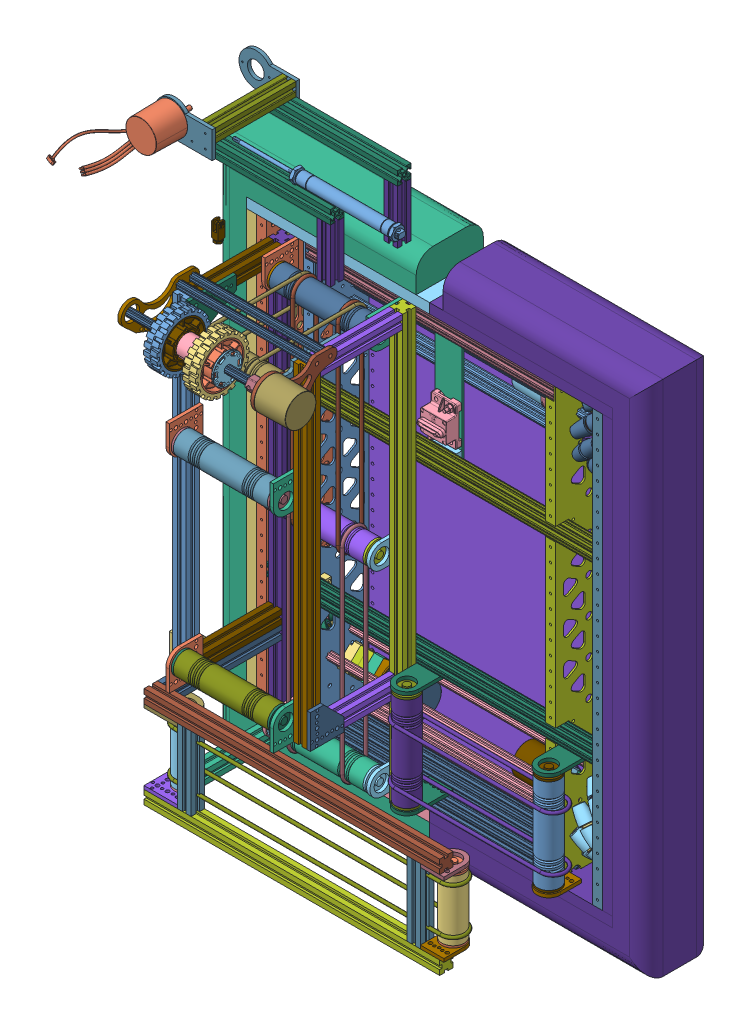
SolidWorks assembly Robot 2020, configuration Default. Lengths in mm. (continued)
Components (placement in the parent): (continued)
- Robot 2020(2)^Robot 2020-1: Robot 2020(2)^Robot 2020 [Default] at origin size (819.15 992.53 549) (virtual) (continued)
  - Fame 2020^Robot 2020(2)_Robot 2020-1: Fame 2020^Robot 2020(2)_Robot 2020 [Default] at origin size (819.15 977.9 171.99) (virtual) (continued)
    - Left Wheel Assembly v4(Mirror)^Fame 2020_Robot 2020(2)_Robot 2020-1: Left Wheel Assembly v4(Mirror)^Fame 2020_Robot 2020(2)_Robot 2020 [Default] at (-500 0 0) x (-1 0 0) z (0 0 -1) size (65.82 166.11 165.01) (virtual) (continued)
      - 6_Mecanum_Wheel_Left_217-2799 v1(Mirror)^Left Wheel Assembly v4(Mirror)_Fame 2020_Robot 2020(2)_Robot 2020-1: 6_Mecanum_Wheel_Left_217-2799 v1(Mirror)^Left Wheel Assembly v4(Mirror)_Fame 2020_Robot 2020(2)_Robot 2020 [Default] x (0 0 -1) z (1 0 0) size (165.01 166.11 65.82) (virtual) (continued)
        - 217-2586-004 Rev1(Mirror)^6_Mecanum_Wheel_Left_217-2799 v1(Mirror)_Left Wheel Assembly v4(Mirror)_Fame 2020_Robot 2020(2)_Robot 2020-6: 217-2586-004 Rev1(Mirror)^6_Mecanum_Wheel_Left_217-2799 v1(Mirror)_Left Wheel Assembly v4(Mirror)_Fame 2020_Robot 2020(2)_Robot 2020 [Default] at (43.5263 -256.0729 -227.2551) x (-0.488796 0.647964 0.584142) z (-0.522795 -0.753596 0.39847) size (25.9 28.58 25.9) (virtual)
        - 217-2586-004 Rev1(Mirror)^6_Mecanum_Wheel_Left_217-2799 v1(Mirror)_Left Wheel Assembly v4(Mirror)_Fame 2020_Robot 2020(2)_Robot 2020-7: 217-2586-004 Rev1(Mirror)^6_Mecanum_Wheel_Left_217-2799 v1(Mirror)_Left Wheel Assembly v4(Mirror)_Fame 2020_Robot 2020(2)_Robot 2020 [Default] at (77.6959 -273.7639 -227.2551) x (-0.01458 0.811521 0.584142) z (-0.865903 -0.302381 0.39847) size (25.9 28.58 25.9) (virtual)
        - 217-2586-004 Rev1(Mirror)^6_Mecanum_Wheel_Left_217-2799 v1(Mirror)_Left Wheel Assembly v4(Mirror)_Fame 2020_Robot 2020(2)_Robot 2020-8: 217-2586-004 Rev1(Mirror)^6_Mecanum_Wheel_Left_217-2799 v1(Mirror)_Left Wheel Assembly v4(Mirror)_Fame 2020_Robot 2020(2)_Robot 2020 [Default] at (94.9412 -308.1606 -227.2551) x (0.465204 0.665104 0.584142) z (-0.878265 0.264334 0.39847) size (25.9 28.58 25.9) (virtual)
        - 217-2586-004 Rev1(Mirror)^6_Mecanum_Wheel_Left_217-2799 v1(Mirror)_Left Wheel Assembly v4(Mirror)_Fame 2020_Robot 2020(2)_Robot 2020-9: 217-2586-004 Rev1(Mirror)^6_Mecanum_Wheel_Left_217-2799 v1(Mirror)_Left Wheel Assembly v4(Mirror)_Fame 2020_Robot 2020(2)_Robot 2020 [Default] at (88.675 -346.1246 -227.2551) x (0.767297 0.26464 0.584142) z (-0.55516 0.730082 0.39847) size (25.9 28.58 25.9) (virtual)
        - 217-2586-004 Rev1(Mirror)^6_Mecanum_Wheel_Left_217-2799 v1(Mirror)_Left Wheel Assembly v4(Mirror)_Fame 2020_Robot 2020(2)_Robot 2020-10: 217-2586-004 Rev1(Mirror)^6_Mecanum_Wheel_Left_217-2799 v1(Mirror)_Left Wheel Assembly v4(Mirror)_Fame 2020_Robot 2020(2)_Robot 2020 [Default] at (61.291 -373.155 -227.2551) x (0.776308 -0.236907 0.584142) z (-0.020002 0.916963 0.39847) size (25.9 28.58 25.9) (virtual)
        - 217-2586-004 Rev1(Mirror)^6_Mecanum_Wheel_Left_217-2799 v1(Mirror)_Left Wheel Assembly v4(Mirror)_Fame 2020_Robot 2020(2)_Robot 2020-11: 217-2586-004 Rev1(Mirror)^6_Mecanum_Wheel_Left_217-2799 v1(Mirror)_Left Wheel Assembly v4(Mirror)_Fame 2020_Robot 2020(2)_Robot 2020 [Default] at (23.2487 -378.9271 -227.2551) x (0.488796 -0.647964 0.584142) z (0.522795 0.753596 0.39847) size (25.9 28.58 25.9) (virtual)
        - 217-2586-004 Rev1(Mirror)^6_Mecanum_Wheel_Left_217-2799 v1(Mirror)_Left Wheel Assembly v4(Mirror)_Fame 2020_Robot 2020(2)_Robot 2020-12: 217-2586-004 Rev1(Mirror)^6_Mecanum_Wheel_Left_217-2799 v1(Mirror)_Left Wheel Assembly v4(Mirror)_Fame 2020_Robot 2020(2)_Robot 2020 [Default] at (-28.0394 -327.6397 -228.0654) x (-0.983582 -0.179 0.02293) z (-0.142587 0.692961 -0.706735) size (25.9 28.58 25.9) (virtual)
        - 217-2586-004 Rev1(Mirror)^6_Mecanum_Wheel_Left_217-2799 v1(Mirror)_Left Wheel Assembly v4(Mirror)_Fame 2020_Robot 2020(2)_Robot 2020-13: 217-2586-004 Rev1(Mirror)^6_Mecanum_Wheel_Left_217-2799 v1(Mirror)_Left Wheel Assembly v4(Mirror)_Fame 2020_Robot 2020(2)_Robot 2020 [Default] at (-22.2679 -289.5974 -228.0654) x (-0.900948 0.433321 0.02293) z (0.291957 0.644427 -0.706735) size (25.9 28.58 25.9) (virtual)
        - 217-2586-004 Rev1(Mirror)^6_Mecanum_Wheel_Left_217-2799 v1(Mirror)_Left Wheel Assembly v4(Mirror)_Fame 2020_Robot 2020(2)_Robot 2020-14: 217-2586-004 Rev1(Mirror)^6_Mecanum_Wheel_Left_217-2799 v1(Mirror)_Left Wheel Assembly v4(Mirror)_Fame 2020_Robot 2020(2)_Robot 2020 [Default] at (4.7621 -262.2129 -228.0654) x (-0.474183 0.880128 0.02293) z (0.614983 0.349745 -0.706735) size (25.9 28.58 25.9) (virtual)
        - 217-2586-004 Rev1(Mirror)^6_Mecanum_Wheel_Left_217-2799 v1(Mirror)_Left Wheel Assembly v4(Mirror)_Fame 2020_Robot 2020(2)_Robot 2020-15: 217-2586-004 Rev1(Mirror)^6_Mecanum_Wheel_Left_217-2799 v1(Mirror)_Left Wheel Assembly v4(Mirror)_Fame 2020_Robot 2020(2)_Robot 2020 [Default] at (42.726 -255.9462 -228.0654) x (0.133704 0.990756 0.02293) z (0.703107 -0.078529 -0.706735) size (25.9 28.58 25.9) (virtual)
        - 217-2586-004 Rev1(Mirror)^6_Mecanum_Wheel_Left_217-2799 v1(Mirror)_Left Wheel Assembly v4(Mirror)_Fame 2020_Robot 2020(2)_Robot 2020-16: 217-2586-004 Rev1(Mirror)^6_Mecanum_Wheel_Left_217-2799 v1(Mirror)_Left Wheel Assembly v4(Mirror)_Fame 2020_Robot 2020(2)_Robot 2020 [Default] at (77.1229 -273.191 -228.0654) x (0.690521 0.722949 0.02293) z (0.522667 -0.476807 -0.706735) size (25.9 28.58 25.9) (virtual)
        - 217-2586-004 Rev1(Mirror)^6_Mecanum_Wheel_Left_217-2799 v1(Mirror)_Left Wheel Assembly v4(Mirror)_Fame 2020_Robot 2020(2)_Robot 2020-17: 217-2586-004 Rev1(Mirror)^6_Mecanum_Wheel_Left_217-2799 v1(Mirror)_Left Wheel Assembly v4(Mirror)_Fame 2020_Robot 2020(2)_Robot 2020 [Default] at (94.8144 -307.3603 -228.0654) x (0.983582 0.179 0.02293) z (0.142587 -0.692961 -0.706735) size (25.9 28.58 25.9) (virtual)
        - 217-2586-004 Rev1(Mirror)^6_Mecanum_Wheel_Left_217-2799 v1(Mirror)_Left Wheel Assembly v4(Mirror)_Fame 2020_Robot 2020(2)_Robot 2020-18: 217-2586-004 Rev1(Mirror)^6_Mecanum_Wheel_Left_217-2799 v1(Mirror)_Left Wheel Assembly v4(Mirror)_Fame 2020_Robot 2020(2)_Robot 2020 [Default] at (89.0429 -345.4026 -228.0654) x (0.900948 -0.433321 0.02293) z (-0.291957 -0.644427 -0.706735) size (25.9 28.58 25.9) (virtual)
        - 217-2586-004 Rev1(Mirror)^6_Mecanum_Wheel_Left_217-2799 v1(Mirror)_Left Wheel Assembly v4(Mirror)_Fame 2020_Robot 2020(2)_Robot 2020-19: 217-2586-004 Rev1(Mirror)^6_Mecanum_Wheel_Left_217-2799 v1(Mirror)_Left Wheel Assembly v4(Mirror)_Fame 2020_Robot 2020(2)_Robot 2020 [Default] at (62.0129 -372.7871 -228.0654) x (0.474183 -0.880128 0.02293) z (-0.614983 -0.349745 -0.706735) size (25.9 28.58 25.9) (virtual)
        - 217-2586-004 Rev1(Mirror)^6_Mecanum_Wheel_Left_217-2799 v1(Mirror)_Left Wheel Assembly v4(Mirror)_Fame 2020_Robot 2020(2)_Robot 2020-20: 217-2586-004 Rev1(Mirror)^6_Mecanum_Wheel_Left_217-2799 v1(Mirror)_Left Wheel Assembly v4(Mirror)_Fame 2020_Robot 2020(2)_Robot 2020 [Default] at (24.049 -379.0538 -228.0654) x (-0.133704 -0.990756 0.02293) z (-0.703107 0.078529 -0.706735) size (25.9 28.58 25.9) (virtual)
        - 217-2586-007 Rev1(Mirror)^6_Mecanum_Wheel_Left_217-2799 v1(Mirror)_Left Wheel Assembly v4(Mirror)_Fame 2020_Robot 2020(2)_Robot 2020-1: 217-2586-007 Rev1(Mirror)^6_Mecanum_Wheel_Left_217-2799 v1(Mirror)_Left Wheel Assembly v4(Mirror)_Fame 2020_Robot 2020(2)_Robot 2020 [Default] at (-10.6347 -361.5222 -227.6598) x (0.5 -0.5 -0.707107) z (0.709055 0.705148 0.002763) size (61.72 5 5) (virtual)
        - 217-2586-007 Rev1(Mirror)^6_Mecanum_Wheel_Left_217-2799 v1(Mirror)_Left Wheel Assembly v4(Mirror)_Fame 2020_Robot 2020(2)_Robot 2020-2: 217-2586-007 Rev1(Mirror)^6_Mecanum_Wheel_Left_217-2799 v1(Mirror)_Left Wheel Assembly v4(Mirror)_Fame 2020_Robot 2020(2)_Robot 2020 [Default] at (-28.1029 -327.2391 -227.6598) x (0.110616 -0.698401 -0.707107) z (0.988113 0.153705 0.002763) size (61.72 5 5) (virtual)
        - 217-2586-007 Rev1(Mirror)^6_Mecanum_Wheel_Left_217-2799 v1(Mirror)_Left Wheel Assembly v4(Mirror)_Fame 2020_Robot 2020(2)_Robot 2020-3: 217-2586-007 Rev1(Mirror)^6_Mecanum_Wheel_Left_217-2799 v1(Mirror)_Left Wheel Assembly v4(Mirror)_Fame 2020_Robot 2020(2)_Robot 2020 [Default] at (-22.0838 -289.236 -227.6598) x (-0.32102 -0.630037 -0.707107) z (0.889746 -0.456448 0.002763) size (61.72 5 5) (virtual)
        - 217-2586-007 Rev1(Mirror)^6_Mecanum_Wheel_Left_217-2799 v1(Mirror)_Left Wheel Assembly v4(Mirror)_Fame 2020_Robot 2020(2)_Robot 2020-4: 217-2586-007 Rev1(Mirror)^6_Mecanum_Wheel_Left_217-2799 v1(Mirror)_Left Wheel Assembly v4(Mirror)_Fame 2020_Robot 2020(2)_Robot 2020 [Default] at (5.1235 -262.0287 -227.6598) x (-0.630037 -0.32102 -0.707107) z (0.451526 -0.892254 0.002763) size (61.72 5 5) (virtual)
        - 217-2586-007 Rev1(Mirror)^6_Mecanum_Wheel_Left_217-2799 v1(Mirror)_Left Wheel Assembly v4(Mirror)_Fame 2020_Robot 2020(2)_Robot 2020-5: 217-2586-007 Rev1(Mirror)^6_Mecanum_Wheel_Left_217-2799 v1(Mirror)_Left Wheel Assembly v4(Mirror)_Fame 2020_Robot 2020(2)_Robot 2020 [Default] at (43.1266 -256.0096 -227.6598) x (-0.698401 0.110616 -0.707107) z (-0.159162 -0.987249 0.002763) size (61.72 5 5) (virtual)
        - 217-2586-007 Rev1(Mirror)^6_Mecanum_Wheel_Left_217-2799 v1(Mirror)_Left Wheel Assembly v4(Mirror)_Fame 2020_Robot 2020(2)_Robot 2020-6: 217-2586-007 Rev1(Mirror)^6_Mecanum_Wheel_Left_217-2799 v1(Mirror)_Left Wheel Assembly v4(Mirror)_Fame 2020_Robot 2020(2)_Robot 2020 [Default] at (77.4097 -273.4778 -227.6598) x (-0.5 0.5 -0.707107) z (-0.709055 -0.705148 0.002763) size (61.72 5 5) (virtual)
        - 217-2586-007 Rev1(Mirror)^6_Mecanum_Wheel_Left_217-2799 v1(Mirror)_Left Wheel Assembly v4(Mirror)_Fame 2020_Robot 2020(2)_Robot 2020-7: 217-2586-007 Rev1(Mirror)^6_Mecanum_Wheel_Left_217-2799 v1(Mirror)_Left Wheel Assembly v4(Mirror)_Fame 2020_Robot 2020(2)_Robot 2020 [Default] at (94.8779 -307.7609 -227.6598) x (-0.110616 0.698401 -0.707107) z (-0.988113 -0.153705 0.002763) size (61.72 5 5) (virtual)
        - 217-2586-007 Rev1(Mirror)^6_Mecanum_Wheel_Left_217-2799 v1(Mirror)_Left Wheel Assembly v4(Mirror)_Fame 2020_Robot 2020(2)_Robot 2020-8: 217-2586-007 Rev1(Mirror)^6_Mecanum_Wheel_Left_217-2799 v1(Mirror)_Left Wheel Assembly v4(Mirror)_Fame 2020_Robot 2020(2)_Robot 2020 [Default] at (88.8588 -345.764 -227.6598) x (0.32102 0.630037 -0.707107) z (-0.889746 0.456448 0.002763) size (61.72 5 5) (virtual)
        - 217-2586-007 Rev1(Mirror)^6_Mecanum_Wheel_Left_217-2799 v1(Mirror)_Left Wheel Assembly v4(Mirror)_Fame 2020_Robot 2020(2)_Robot 2020-9: 217-2586-007 Rev1(Mirror)^6_Mecanum_Wheel_Left_217-2799 v1(Mirror)_Left Wheel Assembly v4(Mirror)_Fame 2020_Robot 2020(2)_Robot 2020 [Default] at (61.6515 -372.9713 -227.6598) x (0.630037 0.32102 -0.707107) z (-0.451526 0.892254 0.002763) size (61.72 5 5) (virtual)
        - 217-2586-007 Rev1(Mirror)^6_Mecanum_Wheel_Left_217-2799 v1(Mirror)_Left Wheel Assembly v4(Mirror)_Fame 2020_Robot 2020(2)_Robot 2020-10: 217-2586-007 Rev1(Mirror)^6_Mecanum_Wheel_Left_217-2799 v1(Mirror)_Left Wheel Assembly v4(Mirror)_Fame 2020_Robot 2020(2)_Robot 2020 [Default] at (23.6484 -378.9904 -227.6598) x (0.698401 -0.110616 -0.707107) z (0.159162 0.987249 0.002763) size (61.72 5 5) (virtual)
        - 217-2586-008 Rev1(Mirror)^6_Mecanum_Wheel_Left_217-2799 v1(Mirror)_Left Wheel Assembly v4(Mirror)_Fame 2020_Robot 2020(2)_Robot 2020-1: 217-2586-008 Rev1(Mirror)^6_Mecanum_Wheel_Left_217-2799 v1(Mirror)_Left Wheel Assembly v4(Mirror)_Fame 2020_Robot 2020(2)_Robot 2020 [Default] at (53.3583 -330.4692 -227.5328) x (0.544639 0.838671 0) z (0 0 -1) size (7.33 6.35 31.75) (virtual)
        - 217-2586-008 Rev1(Mirror)^6_Mecanum_Wheel_Left_217-2799 v1(Mirror)_Left Wheel Assembly v4(Mirror)_Fame 2020_Robot 2020(2)_Robot 2020-2: 217-2586-008 Rev1(Mirror)^6_Mecanum_Wheel_Left_217-2799 v1(Mirror)_Left Wheel Assembly v4(Mirror)_Fame 2020_Robot 2020(2)_Robot 2020 [Default] at (32.1413 -341.2799 -227.5328) x (0.99863 -0.052336 0) z (0 0 -1) size (7.33 6.35 31.75) (virtual)
        - 217-2586-008 Rev1(Mirror)^6_Mecanum_Wheel_Left_217-2799 v1(Mirror)_Left Wheel Assembly v4(Mirror)_Fame 2020_Robot 2020(2)_Robot 2020-3: 217-2586-008 Rev1(Mirror)^6_Mecanum_Wheel_Left_217-2799 v1(Mirror)_Left Wheel Assembly v4(Mirror)_Fame 2020_Robot 2020(2)_Robot 2020 [Default] at (12.1704 -328.3106 -227.5328) x (0.45399 -0.891007 0) z (0 0 -1) size (7.33 6.35 31.75) (virtual)
        - 217-2586-008 Rev1(Mirror)^6_Mecanum_Wheel_Left_217-2799 v1(Mirror)_Left Wheel Assembly v4(Mirror)_Fame 2020_Robot 2020(2)_Robot 2020-4: 217-2586-008 Rev1(Mirror)^6_Mecanum_Wheel_Left_217-2799 v1(Mirror)_Left Wheel Assembly v4(Mirror)_Fame 2020_Robot 2020(2)_Robot 2020 [Default] at (13.4167 -304.5308 -227.5328) x (-0.544639 -0.838671 0) z (0 0 -1) size (7.33 6.35 31.75) (virtual)
        - 217-2586-008 Rev1(Mirror)^6_Mecanum_Wheel_Left_217-2799 v1(Mirror)_Left Wheel Assembly v4(Mirror)_Fame 2020_Robot 2020(2)_Robot 2020-5: 217-2586-008 Rev1(Mirror)^6_Mecanum_Wheel_Left_217-2799 v1(Mirror)_Left Wheel Assembly v4(Mirror)_Fame 2020_Robot 2020(2)_Robot 2020 [Default] at (34.6337 -293.7201 -227.5328) x (-0.99863 0.052336 0) z (0 0 -1) size (7.33 6.35 31.75) (virtual)
        - 217-2586-008 Rev1(Mirror)^6_Mecanum_Wheel_Left_217-2799 v1(Mirror)_Left Wheel Assembly v4(Mirror)_Fame 2020_Robot 2020(2)_Robot 2020-6: 217-2586-008 Rev1(Mirror)^6_Mecanum_Wheel_Left_217-2799 v1(Mirror)_Left Wheel Assembly v4(Mirror)_Fame 2020_Robot 2020(2)_Robot 2020 [Default] at (54.6046 -306.6894 -227.5328) x (-0.45399 0.891007 0) z (0 0 -1) size (7.33 6.35 31.75) (virtual)
        - NUT-832-NYLOCK(Mirror)^6_Mecanum_Wheel_Left_217-2799 v1(Mirror)_Left Wheel Assembly v4(Mirror)_Fame 2020_Robot 2020(2)_Robot 2020-1: NUT-832-NYLOCK(Mirror)^6_Mecanum_Wheel_Left_217-2799 v1(Mirror)_Left Wheel Assembly v4(Mirror)_Fame 2020_Robot 2020(2)_Robot 2020 [Default] at (6.1639 -290.2764 -241.3161) x (0.258819 -0.965926 0) z (0.965926 0.258819 0) size (9.37 5.86 8.12) (virtual)
        - NUT-832-NYLOCK(Mirror)^6_Mecanum_Wheel_Left_217-2799 v1(Mirror)_Left Wheel Assembly v4(Mirror)_Fame 2020_Robot 2020(2)_Robot 2020-2: NUT-832-NYLOCK(Mirror)^6_Mecanum_Wheel_Left_217-2799 v1(Mirror)_Left Wheel Assembly v4(Mirror)_Fame 2020_Robot 2020(2)_Robot 2020 [Default] at (-0.9163 -334.9786 -241.3161) x (0.99863 -0.052336 0) z (0.052336 0.99863 0) size (9.37 5.86 8.12) (virtual)
        - NUT-832-NYLOCK(Mirror)^6_Mecanum_Wheel_Left_217-2799 v1(Mirror)_Left Wheel Assembly v4(Mirror)_Fame 2020_Robot 2020(2)_Robot 2020-3: NUT-832-NYLOCK(Mirror)^6_Mecanum_Wheel_Left_217-2799 v1(Mirror)_Left Wheel Assembly v4(Mirror)_Fame 2020_Robot 2020(2)_Robot 2020 [Default] at (39.4102 -355.526 -241.3161) x (0.358368 0.93358 0) z (-0.93358 0.358368 0) size (9.37 5.86 8.12) (virtual)
        - NUT-832-NYLOCK(Mirror)^6_Mecanum_Wheel_Left_217-2799 v1(Mirror)_Left Wheel Assembly v4(Mirror)_Fame 2020_Robot 2020(2)_Robot 2020-4: NUT-832-NYLOCK(Mirror)^6_Mecanum_Wheel_Left_217-2799 v1(Mirror)_Left Wheel Assembly v4(Mirror)_Fame 2020_Robot 2020(2)_Robot 2020 [Default] at (71.4135 -323.5227 -241.3161) x (-0.777146 0.62932 0) z (-0.62932 -0.777146 0) size (9.37 5.86 8.12) (virtual)
        - NUT-832-NYLOCK(Mirror)^6_Mecanum_Wheel_Left_217-2799 v1(Mirror)_Left Wheel Assembly v4(Mirror)_Fame 2020_Robot 2020(2)_Robot 2020-5: NUT-832-NYLOCK(Mirror)^6_Mecanum_Wheel_Left_217-2799 v1(Mirror)_Left Wheel Assembly v4(Mirror)_Fame 2020_Robot 2020(2)_Robot 2020 [Default] at (50.8661 -283.1962 -241.3161) x (-0.838671 -0.544639 0) z (0.544639 -0.838671 0) size (9.37 5.86 8.12) (virtual)
        - SCREW-832-1250(Mirror)^6_Mecanum_Wheel_Left_217-2799 v1(Mirror)_Left Wheel Assembly v4(Mirror)_Fame 2020_Robot 2020(2)_Robot 2020-1: SCREW-832-1250(Mirror)^6_Mecanum_Wheel_Left_217-2799 v1(Mirror)_Left Wheel Assembly v4(Mirror)_Fame 2020_Robot 2020(2)_Robot 2020 [Default] at (6.1639 -290.2764 -212.75) x (0 0 -1) z (0.394243 -0.919006 0) size (33.96 7.92 7.92) (virtual)
        - SCREW-832-1250(Mirror)^6_Mecanum_Wheel_Left_217-2799 v1(Mirror)_Left Wheel Assembly v4(Mirror)_Fame 2020_Robot 2020(2)_Robot 2020-2: SCREW-832-1250(Mirror)^6_Mecanum_Wheel_Left_217-2799 v1(Mirror)_Left Wheel Assembly v4(Mirror)_Fame 2020_Robot 2020(2)_Robot 2020 [Default] at (-0.9163 -334.9786 -212.75) x (0 0 -1) z (0.995855 0.090959 0) size (33.96 7.92 7.92) (virtual)
        - SCREW-832-1250(Mirror)^6_Mecanum_Wheel_Left_217-2799 v1(Mirror)_Left Wheel Assembly v4(Mirror)_Fame 2020_Robot 2020(2)_Robot 2020-3: SCREW-832-1250(Mirror)^6_Mecanum_Wheel_Left_217-2799 v1(Mirror)_Left Wheel Assembly v4(Mirror)_Fame 2020_Robot 2020(2)_Robot 2020 [Default] at (39.4102 -355.526 -212.75) x (0 0 -1) z (0.221229 0.975222 0) size (33.96 7.92 7.92) (virtual)
        - SCREW-832-1250(Mirror)^6_Mecanum_Wheel_Left_217-2799 v1(Mirror)_Left Wheel Assembly v4(Mirror)_Fame 2020_Robot 2020(2)_Robot 2020-4: SCREW-832-1250(Mirror)^6_Mecanum_Wheel_Left_217-2799 v1(Mirror)_Left Wheel Assembly v4(Mirror)_Fame 2020_Robot 2020(2)_Robot 2020 [Default] at (71.4135 -323.5227 -212.75) x (0 0 -1) z (-0.859128 0.511761 0) size (33.96 7.92 7.92) (virtual)
        - SCREW-832-1250(Mirror)^6_Mecanum_Wheel_Left_217-2799 v1(Mirror)_Left Wheel Assembly v4(Mirror)_Fame 2020_Robot 2020(2)_Robot 2020-5: SCREW-832-1250(Mirror)^6_Mecanum_Wheel_Left_217-2799 v1(Mirror)_Left Wheel Assembly v4(Mirror)_Fame 2020_Robot 2020(2)_Robot 2020 [Default] at (50.8661 -283.1962 -212.75) x (0 0 -1) z (-0.752199 -0.658936 0) size (33.96 7.92 7.92) (virtual)
        - 217-2586-005 Rev2(Mirror)^6_Mecanum_Wheel_Left_217-2799 v1(Mirror)_Left Wheel Assembly v4(Mirror)_Fame 2020_Robot 2020(2)_Robot 2020-1: 217-2586-005 Rev2(Mirror)^6_Mecanum_Wheel_Left_217-2799 v1(Mirror)_Left Wheel Assembly v4(Mirror)_Fame 2020_Robot 2020(2)_Robot 2020 [Default] at (-6.1597 -365.9972 -233.9884) x (-0.5 0.5 0.707107) z (-0.146447 -0.853553 0.5) size (8.5 8 8) (virtual)
        - 217-2586-005 Rev2(Mirror)^6_Mecanum_Wheel_Left_217-2799 v1(Mirror)_Left Wheel Assembly v4(Mirror)_Fame 2020_Robot 2020(2)_Robot 2020-2: 217-2586-005 Rev2(Mirror)^6_Mecanum_Wheel_Left_217-2799 v1(Mirror)_Left Wheel Assembly v4(Mirror)_Fame 2020_Robot 2020(2)_Robot 2020 [Default] at (-15.1097 -357.0472 -221.3312) x (-0.5 0.5 0.707107) z (-0.146447 -0.853553 0.5) size (8.5 8 8) (virtual)
        - 217-2586-005 Rev2(Mirror)^6_Mecanum_Wheel_Left_217-2799 v1(Mirror)_Left Wheel Assembly v4(Mirror)_Fame 2020_Robot 2020(2)_Robot 2020-3: 217-2586-005 Rev2(Mirror)^6_Mecanum_Wheel_Left_217-2799 v1(Mirror)_Left Wheel Assembly v4(Mirror)_Fame 2020_Robot 2020(2)_Robot 2020 [Default] at (-29.0929 -320.9884 -221.3312) x (-0.110616 0.698401 0.707107) z (-0.620184 -0.60446 0.5) size (8.5 8 8) (virtual)
        - 217-2586-005 Rev2(Mirror)^6_Mecanum_Wheel_Left_217-2799 v1(Mirror)_Left Wheel Assembly v4(Mirror)_Fame 2020_Robot 2020(2)_Robot 2020-4: 217-2586-005 Rev2(Mirror)^6_Mecanum_Wheel_Left_217-2799 v1(Mirror)_Left Wheel Assembly v4(Mirror)_Fame 2020_Robot 2020(2)_Robot 2020 [Default] at (-19.2106 -283.5972 -221.3312) x (0.32102 0.630037 0.707107) z (-0.857032 -0.124484 0.5) size (8.5 8 8) (virtual)
        - 217-2586-005 Rev2(Mirror)^6_Mecanum_Wheel_Left_217-2799 v1(Mirror)_Left Wheel Assembly v4(Mirror)_Fame 2020_Robot 2020(2)_Robot 2020-5: 217-2586-005 Rev2(Mirror)^6_Mecanum_Wheel_Left_217-2799 v1(Mirror)_Left Wheel Assembly v4(Mirror)_Fame 2020_Robot 2020(2)_Robot 2020 [Default] at (10.7623 -259.1556 -221.3312) x (0.630037 0.32102 0.707107) z (-0.766523 0.403042 0.5) size (8.5 8 8) (virtual)
        - 217-2586-005 Rev2(Mirror)^6_Mecanum_Wheel_Left_217-2799 v1(Mirror)_Left Wheel Assembly v4(Mirror)_Fame 2020_Robot 2020(2)_Robot 2020-6: 217-2586-005 Rev2(Mirror)^6_Mecanum_Wheel_Left_217-2799 v1(Mirror)_Left Wheel Assembly v4(Mirror)_Fame 2020_Robot 2020(2)_Robot 2020 [Default] at (49.3773 -256.9997 -221.3312) x (0.698401 -0.110616 0.707107) z (-0.383228 0.776618 0.5) size (8.5 8 8) (virtual)
        - 217-2586-005 Rev2(Mirror)^6_Mecanum_Wheel_Left_217-2799 v1(Mirror)_Left Wheel Assembly v4(Mirror)_Fame 2020_Robot 2020(2)_Robot 2020-7: 217-2586-005 Rev2(Mirror)^6_Mecanum_Wheel_Left_217-2799 v1(Mirror)_Left Wheel Assembly v4(Mirror)_Fame 2020_Robot 2020(2)_Robot 2020 [Default] at (81.8847 -277.9528 -221.3312) x (0.5 -0.5 0.707107) z (0.146447 0.853553 0.5) size (8.5 8 8) (virtual)
        - 217-2586-005 Rev2(Mirror)^6_Mecanum_Wheel_Left_217-2799 v1(Mirror)_Left Wheel Assembly v4(Mirror)_Fame 2020_Robot 2020(2)_Robot 2020-8: 217-2586-005 Rev2(Mirror)^6_Mecanum_Wheel_Left_217-2799 v1(Mirror)_Left Wheel Assembly v4(Mirror)_Fame 2020_Robot 2020(2)_Robot 2020 [Default] at (95.8679 -314.0116 -221.3312) x (0.110616 -0.698401 0.707107) z (0.620184 0.60446 0.5) size (8.5 8 8) (virtual)
        - 217-2586-005 Rev2(Mirror)^6_Mecanum_Wheel_Left_217-2799 v1(Mirror)_Left Wheel Assembly v4(Mirror)_Fame 2020_Robot 2020(2)_Robot 2020-9: 217-2586-005 Rev2(Mirror)^6_Mecanum_Wheel_Left_217-2799 v1(Mirror)_Left Wheel Assembly v4(Mirror)_Fame 2020_Robot 2020(2)_Robot 2020 [Default] at (85.9856 -351.4028 -221.3312) x (-0.32102 -0.630037 0.707107) z (0.857032 0.124484 0.5) size (8.5 8 8) (virtual)
        - 217-2586-005 Rev2(Mirror)^6_Mecanum_Wheel_Left_217-2799 v1(Mirror)_Left Wheel Assembly v4(Mirror)_Fame 2020_Robot 2020(2)_Robot 2020-10: 217-2586-005 Rev2(Mirror)^6_Mecanum_Wheel_Left_217-2799 v1(Mirror)_Left Wheel Assembly v4(Mirror)_Fame 2020_Robot 2020(2)_Robot 2020 [Default] at (56.0127 -375.8444 -221.3312) x (-0.630037 -0.32102 0.707107) z (0.766523 -0.403042 0.5) size (8.5 8 8) (virtual)
        - 217-2586-005 Rev2(Mirror)^6_Mecanum_Wheel_Left_217-2799 v1(Mirror)_Left Wheel Assembly v4(Mirror)_Fame 2020_Robot 2020(2)_Robot 2020-11: 217-2586-005 Rev2(Mirror)^6_Mecanum_Wheel_Left_217-2799 v1(Mirror)_Left Wheel Assembly v4(Mirror)_Fame 2020_Robot 2020(2)_Robot 2020 [Default] at (17.3977 -378.0003 -221.3312) x (-0.698401 0.110616 0.707107) z (0.383228 -0.776618 0.5) size (8.5 8 8) (virtual)
        - 217-2586-005 Rev2(Mirror)^6_Mecanum_Wheel_Left_217-2799 v1(Mirror)_Left Wheel Assembly v4(Mirror)_Fame 2020_Robot 2020(2)_Robot 2020-12: 217-2586-005 Rev2(Mirror)^6_Mecanum_Wheel_Left_217-2799 v1(Mirror)_Left Wheel Assembly v4(Mirror)_Fame 2020_Robot 2020(2)_Robot 2020 [Default] at (-27.1128 -333.4898 -233.9884) x (-0.110616 0.698401 0.707107) z (-0.620184 -0.60446 0.5) size (8.5 8 8) (virtual)
        - 217-2586-005 Rev2(Mirror)^6_Mecanum_Wheel_Left_217-2799 v1(Mirror)_Left Wheel Assembly v4(Mirror)_Fame 2020_Robot 2020(2)_Robot 2020-13: 217-2586-005 Rev2(Mirror)^6_Mecanum_Wheel_Left_217-2799 v1(Mirror)_Left Wheel Assembly v4(Mirror)_Fame 2020_Robot 2020(2)_Robot 2020 [Default] at (-24.9569 -294.8748 -233.9884) x (0.32102 0.630037 0.707107) z (-0.857032 -0.124484 0.5) size (8.5 8 8) (virtual)
        - 217-2586-005 Rev2(Mirror)^6_Mecanum_Wheel_Left_217-2799 v1(Mirror)_Left Wheel Assembly v4(Mirror)_Fame 2020_Robot 2020(2)_Robot 2020-14: 217-2586-005 Rev2(Mirror)^6_Mecanum_Wheel_Left_217-2799 v1(Mirror)_Left Wheel Assembly v4(Mirror)_Fame 2020_Robot 2020(2)_Robot 2020 [Default] at (-0.5153 -264.9019 -233.9884) x (0.630037 0.32102 0.707107) z (-0.766523 0.403042 0.5) size (8.5 8 8) (virtual)
        - 217-2586-005 Rev2(Mirror)^6_Mecanum_Wheel_Left_217-2799 v1(Mirror)_Left Wheel Assembly v4(Mirror)_Fame 2020_Robot 2020(2)_Robot 2020-15: 217-2586-005 Rev2(Mirror)^6_Mecanum_Wheel_Left_217-2799 v1(Mirror)_Left Wheel Assembly v4(Mirror)_Fame 2020_Robot 2020(2)_Robot 2020 [Default] at (36.8759 -255.0196 -233.9884) x (0.698401 -0.110616 0.707107) z (-0.383228 0.776618 0.5) size (8.5 8 8) (virtual)
        - 217-2586-005 Rev2(Mirror)^6_Mecanum_Wheel_Left_217-2799 v1(Mirror)_Left Wheel Assembly v4(Mirror)_Fame 2020_Robot 2020(2)_Robot 2020-16: 217-2586-005 Rev2(Mirror)^6_Mecanum_Wheel_Left_217-2799 v1(Mirror)_Left Wheel Assembly v4(Mirror)_Fame 2020_Robot 2020(2)_Robot 2020 [Default] at (72.9347 -269.0028 -233.9884) x (0.5 -0.5 0.707107) z (0.146447 0.853553 0.5) size (8.5 8 8) (virtual)
        - 217-2586-005 Rev2(Mirror)^6_Mecanum_Wheel_Left_217-2799 v1(Mirror)_Left Wheel Assembly v4(Mirror)_Fame 2020_Robot 2020(2)_Robot 2020-17: 217-2586-005 Rev2(Mirror)^6_Mecanum_Wheel_Left_217-2799 v1(Mirror)_Left Wheel Assembly v4(Mirror)_Fame 2020_Robot 2020(2)_Robot 2020 [Default] at (93.8878 -301.5102 -233.9884) x (0.110616 -0.698401 0.707107) z (0.620184 0.60446 0.5) size (8.5 8 8) (virtual)
        - 217-2586-005 Rev2(Mirror)^6_Mecanum_Wheel_Left_217-2799 v1(Mirror)_Left Wheel Assembly v4(Mirror)_Fame 2020_Robot 2020(2)_Robot 2020-18: 217-2586-005 Rev2(Mirror)^6_Mecanum_Wheel_Left_217-2799 v1(Mirror)_Left Wheel Assembly v4(Mirror)_Fame 2020_Robot 2020(2)_Robot 2020 [Default] at (91.7319 -340.1252 -233.9884) x (-0.32102 -0.630037 0.707107) z (0.857032 0.124484 0.5) size (8.5 8 8) (virtual)
        - 217-2586-005 Rev2(Mirror)^6_Mecanum_Wheel_Left_217-2799 v1(Mirror)_Left Wheel Assembly v4(Mirror)_Fame 2020_Robot 2020(2)_Robot 2020-19: 217-2586-005 Rev2(Mirror)^6_Mecanum_Wheel_Left_217-2799 v1(Mirror)_Left Wheel Assembly v4(Mirror)_Fame 2020_Robot 2020(2)_Robot 2020 [Default] at (67.2903 -370.0981 -233.9884) x (-0.630037 -0.32102 0.707107) z (0.766523 -0.403042 0.5) size (8.5 8 8) (virtual)
        - 217-2586-005 Rev2(Mirror)^6_Mecanum_Wheel_Left_217-2799 v1(Mirror)_Left Wheel Assembly v4(Mirror)_Fame 2020_Robot 2020(2)_Robot 2020-20: 217-2586-005 Rev2(Mirror)^6_Mecanum_Wheel_Left_217-2799 v1(Mirror)_Left Wheel Assembly v4(Mirror)_Fame 2020_Robot 2020(2)_Robot 2020 [Default] at (29.8991 -379.9804 -233.9884) x (-0.698401 0.110616 0.707107) z (0.383228 -0.776618 0.5) size (8.5 8 8) (virtual)
      - 1_2_Hex_Bore_Aluminum_VersaHub_217-2592 v1(Mirror)^Left Wheel Assembly v4(Mirror)_Fame 2020_Robot 2020(2)_Robot 2020-1: 1_2_Hex_Bore_Aluminum_VersaHub_217-2592 v1(Mirror)^Left Wheel Assembly v4(Mirror)_Fame 2020_Robot 2020(2)_Robot 2020 [Default] at (-239.7248 -317.5 -33.3875) x (-1 0 0) z (0 -0.707107 0.707107) size (12.7 55.88 55.88) (virtual)
    - Back Electronics Strap^Fame 2020_Robot 2020(2)_Robot 2020-1: Back Electronics Strap^Fame 2020_Robot 2020(2)_Robot 2020 [Default] at (0.05 266.7 84.65) x (0 1 0) z (0 0 1) size (228.6 81.6 66.64) (virtual)
      - am-0282 120a Circuit Breaker^Back Electronics Strap_Fame 2020_Robot 2020(2)_Robot 2020-1: am-0282 120a Circuit Breaker^Back Electronics Strap_Fame 2020_Robot 2020(2)_Robot 2020 [Default] at (-47.625 0 6.4135) x (1 0 0) z (0 -1 0) size (76.93 61.08 66.64) (virtual)
      - Electronics Strap Front Standoff^Back Electronics Strap_Fame 2020_Robot 2020(2)_Robot 2020-1: Electronics Strap Front Standoff^Back Electronics Strap_Fame 2020_Robot 2020(2)_Robot 2020 [Default] at (-101.6 0 7.1437) size (25.4 50.8 11.11) (virtual)
      - Back Electronics Strap-6^Back Electronics Strap_Fame 2020_Robot 2020(2)_Robot 2020-1: Back Electronics Strap-6^Back Electronics Strap_Fame 2020_Robot 2020(2)_Robot 2020 [Default] at origin size (228.6 50.8 3.17) (virtual)
    - Inner plate^Fame 2020_Robot 2020(2)_Robot 2020-1: Inner plate^Fame 2020_Robot 2020(2)_Robot 2020 [Default] at (212.725 0 58.7875) x (0 1 0) z (0 0 1) size (812.8 19.05 127) (virtual)
    - Base Plate^Fame 2020_Robot 2020(2)_Robot 2020-1: Base Plate^Fame 2020_Robot 2020(2)_Robot 2020 [Default] at origin size (469.9 812.8 3.17) (virtual)
    - 2.75_ Churro^Fame 2020_Robot 2020(2)_Robot 2020-1: 2.75_ Churro^Fame 2020_Robot 2020(2)_Robot 2020 [Default] at (238.125 -165.1 7.9875) x (0 0 -1) z (1 0 0) size (14.66 12.7 69.85) (virtual)
    - 1030-CL-16^Fame 2020_Robot 2020(2)_Robot 2020-1: 1030-CL-16^Fame 2020_Robot 2020(2)_Robot 2020 [Default] at (-184.1 -393.7 84.1875) x (0 -1 0) z (-1 0 0) size (25.4 76.2 469.9) (virtual)
    - 2.75_ Churro v1(Mirror) (2)^Fame 2020_Robot 2020(2)_Robot 2020-1: 2.75_ Churro v1(Mirror) (2)^Fame 2020_Robot 2020(2)_Robot 2020 [Default] at (238.125 165.1 7.9875) x (0 0 -1) z (-1 0 0) size (14.66 12.7 69.85) (virtual)
    - 2.75_ Churro v1(Mirror)^Fame 2020_Robot 2020(2)_Robot 2020-1: 2.75_ Churro v1(Mirror)^Fame 2020_Robot 2020(2)_Robot 2020 [Default] at (-238.125 -165.1 7.9875) x (0 0 -1) z (1 0 0) size (14.66 12.7 69.85) (virtual)
    - 1030-CL-16 v2(Mirror)^Fame 2020_Robot 2020(2)_Robot 2020-1: 1030-CL-16 v2(Mirror)^Fame 2020_Robot 2020(2)_Robot 2020 [Default] at (-184.1 393.7 84.1875) x (0 1 0) z (1 0 0) size (25.4 76.2 469.9) (virtual)
    - Outer plate^Fame 2020_Robot 2020(2)_Robot 2020-1: Outer plate^Fame 2020_Robot 2020(2)_Robot 2020 [Default] at (333.375 0 58.7875) x (0 -1 0) z (0 0 1) size (812.8 19.05 127) (virtual)
    - 1010-CL-22^Fame 2020_Robot 2020(2)_Robot 2020-1: 1010-CL-22^Fame 2020_Robot 2020(2)_Robot 2020 [Default] at (-257.175 -165.1 109.5875) x (0 0 1) z (-1 0 0) size (25.4 25.4 615.95) (virtual)
    - 1010-CL-22 v2(Mirror)^Fame 2020_Robot 2020(2)_Robot 2020-1: 1010-CL-22 v2(Mirror)^Fame 2020_Robot 2020(2)_Robot 2020 [Default] at (-257.175 165.1 109.5875) x (0 0 1) z (1 0 0) size (25.4 25.4 615.95) (virtual)
    - Bumper Assembly^Fame 2020_Robot 2020(2)_Robot 2020-1: Bumper Assembly^Fame 2020_Robot 2020(2)_Robot 2020 [Default] at (327.025 0.0665 58.7875) size (409.58 977.9 127) (virtual)
    - Inner Plate Cross Lock v4^Fame 2020_Robot 2020(2)_Robot 2020-1: Inner Plate Cross Lock v4^Fame 2020_Robot 2020(2)_Robot 2020 [Default] at (235 -165.1 96.8875) x (0 1 0) z (0 0 1) size (25.4 12.7 12.7) (virtual)
    - Motor Brace^Fame 2020_Robot 2020(2)_Robot 2020-1: Motor Brace^Fame 2020_Robot 2020(2)_Robot 2020 [Default] at (120.6 292.8812 76.0284) x (0 0 1) z (-1 0 0) size (14.66 12.7 470) (virtual)
    - Inner Plate Cross Lock v4 v1(Mirror) (2)^Fame 2020_Robot 2020(2)_Robot 2020-1: Inner Plate Cross Lock v4 v1(Mirror) (2)^Fame 2020_Robot 2020(2)_Robot 2020 [Default] at (235 165.1 96.8875) x (0 -1 0) z (0 0 -1) size (25.4 12.7 12.7) (virtual)
    - Inner Plate Cross Lock v4 v1(Mirror)^Fame 2020_Robot 2020(2)_Robot 2020-1: Inner Plate Cross Lock v4 v1(Mirror)^Fame 2020_Robot 2020(2)_Robot 2020 [Default] at (-235 -165.1 96.8875) x (0 1 0) z (0 0 -1) size (25.4 12.7 12.7) (virtual)
    - Motor Brace^Fame 2020_Robot 2020(2)_Robot 2020-2: Motor Brace^Fame 2020_Robot 2020(2)_Robot 2020 [Default] at (-69.8 342.1188 76.0284) x (0 0 -1) z (1 0 0) size (14.66 12.7 470) (virtual)
    - Motor Brace^Fame 2020_Robot 2020(2)_Robot 2020-3: Motor Brace^Fame 2020_Robot 2020(2)_Robot 2020 [Default] at (120.6 268.2625 33.3875) x (0 0 1) z (-1 0 0) size (14.66 12.7 470) (virtual)
    - Motor Brace^Fame 2020_Robot 2020(2)_Robot 2020-4: Motor Brace^Fame 2020_Robot 2020(2)_Robot 2020 [Default] at (-69.8 366.7375 33.3875) x (0 0 -1) z (1 0 0) size (14.66 12.7 470) (virtual)
    - Motor Brace v1(Mirror)^Fame 2020_Robot 2020(2)_Robot 2020-1: Motor Brace v1(Mirror)^Fame 2020_Robot 2020(2)_Robot 2020 [Default] at (120.6 -292.8812 76.0284) x (0 0 1) z (1 0 0) size (14.66 12.7 470) (virtual)
    - Motor Brace v1(Mirror)^Fame 2020_Robot 2020(2)_Robot 2020-2: Motor Brace v1(Mirror)^Fame 2020_Robot 2020(2)_Robot 2020 [Default] at (-69.8 -342.1188 76.0284) x (0 0 -1) z (-1 0 0) size (14.66 12.7 470) (virtual)
    - Motor Brace v1(Mirror)^Fame 2020_Robot 2020(2)_Robot 2020-3: Motor Brace v1(Mirror)^Fame 2020_Robot 2020(2)_Robot 2020 [Default] at (120.6 -268.2625 33.3875) x (0 0 1) z (1 0 0) size (14.66 12.7 470) (virtual)
    - Motor Brace v1(Mirror)^Fame 2020_Robot 2020(2)_Robot 2020-4: Motor Brace v1(Mirror)^Fame 2020_Robot 2020(2)_Robot 2020 [Default] at (-69.8 -366.7375 33.3875) x (0 0 -1) z (-1 0 0) size (14.66 12.7 470) (virtual)
  - Snake^Robot 2020(2)_Robot 2020-1: Snake^Robot 2020(2)_Robot 2020 [Default] at (-279.4 -406.4 122.2875) x (0 -1 0) z (0 0 1) size (812.8 266.7 245.82) (virtual)
    - Roller^Snake_Robot 2020(2)_Robot 2020-1: Roller^Snake_Robot 2020(2)_Robot 2020 [Default] at origin size (42.07 200.15 42.07) (virtual)
      - Roller Hub^Roller_Snake_Robot 2020(2)_Robot 2020-1: Roller Hub^Roller_Snake_Robot 2020(2)_Robot 2020 [Default] at (-39.6875 31.75 39.6875) size (42.07 25.4 42.07) (virtual)
      - Roller 7^Roller_Snake_Robot 2020(2)_Robot 2020-1: Roller 7^Roller_Snake_Robot 2020(2)_Robot 2020 [Default] at (-39.6875 125.476 39.6875) size (42.07 177.8 42.07) (virtual)
      - Roller Hub^Roller_Snake_Robot 2020(2)_Robot 2020-2: Roller Hub^Roller_Snake_Robot 2020(2)_Robot 2020 [Default] at (-39.6875 219.202 39.6875) x (1 0 0) z (0 0 -1) size (42.07 25.4 42.07) (virtual)
    - Roller_1^Snake_Robot 2020(2)_Robot 2020-1: Roller_1^Snake_Robot 2020(2)_Robot 2020 [Default] at origin size (42.07 200.15 42.07) (virtual)
      - Roller Hub^Roller_1_Snake_Robot 2020(2)_Robot 2020-1: Roller Hub^Roller_1_Snake_Robot 2020(2)_Robot 2020 [Default] at (-411.1625 31.75 39.6875) size (42.07 25.4 42.07) (virtual)
      - Roller 7^Roller_1_Snake_Robot 2020(2)_Robot 2020-1: Roller 7^Roller_1_Snake_Robot 2020(2)_Robot 2020 [Default] at (-411.1625 125.476 39.6875) size (42.07 177.8 42.07) (virtual)
      - Roller Hub^Roller_1_Snake_Robot 2020(2)_Robot 2020-2: Roller Hub^Roller_1_Snake_Robot 2020(2)_Robot 2020 [Default] at (-411.1625 219.202 39.6875) x (1 0 0) z (0 0 -1) size (42.07 25.4 42.07) (virtual)
    - Roller_2^Snake_Robot 2020(2)_Robot 2020-1: Roller_2^Snake_Robot 2020(2)_Robot 2020 [Default] at origin size (42.07 200.15 42.07) (virtual)
      - Roller Hub^Roller_2_Snake_Robot 2020(2)_Robot 2020-1: Roller Hub^Roller_2_Snake_Robot 2020(2)_Robot 2020 [Default] at (-773.1125 31.75 39.6875) size (42.07 25.4 42.07) (virtual)
      - Roller 7^Roller_2_Snake_Robot 2020(2)_Robot 2020-1: Roller 7^Roller_2_Snake_Robot 2020(2)_Robot 2020 [Default] at (-773.1125 125.476 39.6875) size (42.07 177.8 42.07) (virtual)
      - Roller Hub^Roller_2_Snake_Robot 2020(2)_Robot 2020-2: Roller Hub^Roller_2_Snake_Robot 2020(2)_Robot 2020 [Default] at (-773.1125 219.202 39.6875) x (1 0 0) z (0 0 -1) size (42.07 25.4 42.07) (virtual)
    - Roller_3^Snake_Robot 2020(2)_Robot 2020-1: Roller_3^Snake_Robot 2020(2)_Robot 2020 [Default] at origin size (42.07 200.15 42.07) (virtual)
      - Roller Hub^Roller_3_Snake_Robot 2020(2)_Robot 2020-1: Roller Hub^Roller_3_Snake_Robot 2020(2)_Robot 2020 [Default] at (-773.1125 31.75 220.6625) size (42.07 25.4 42.07) (virtual)
      - Roller 7^Roller_3_Snake_Robot 2020(2)_Robot 2020-1: Roller 7^Roller_3_Snake_Robot 2020(2)_Robot 2020 [Default] at (-773.1125 125.476 220.6625) size (42.07 177.8 42.07) (virtual)
      - Roller Hub^Roller_3_Snake_Robot 2020(2)_Robot 2020-2: Roller Hub^Roller_3_Snake_Robot 2020(2)_Robot 2020 [Default] at (-773.1125 219.202 220.6625) x (1 0 0) z (0 0 -1) size (42.07 25.4 42.07) (virtual)
    - Roller_4^Snake_Robot 2020(2)_Robot 2020-1: Roller_4^Snake_Robot 2020(2)_Robot 2020 [Default] at origin size (42.07 200.15 42.07) (virtual)
      - Roller Hub^Roller_4_Snake_Robot 2020(2)_Robot 2020-1: Roller Hub^Roller_4_Snake_Robot 2020(2)_Robot 2020 [Default] at (-592.1375 31.75 220.6625) size (42.07 25.4 42.07) (virtual)
      - Roller 7^Roller_4_Snake_Robot 2020(2)_Robot 2020-1: Roller 7^Roller_4_Snake_Robot 2020(2)_Robot 2020 [Default] at (-592.1375 125.476 220.6625) size (42.07 177.8 42.07) (virtual)
      - Roller Hub^Roller_4_Snake_Robot 2020(2)_Robot 2020-2: Roller Hub^Roller_4_Snake_Robot 2020(2)_Robot 2020 [Default] at (-592.1375 219.202 220.6625) x (1 0 0) z (0 0 -1) size (42.07 25.4 42.07) (virtual)
    - Roller_5^Snake_Robot 2020(2)_Robot 2020-1: Roller_5^Snake_Robot 2020(2)_Robot 2020 [Default] at origin size (42.07 200.15 42.07) (virtual)
      - Roller Hub^Roller_5_Snake_Robot 2020(2)_Robot 2020-1: Roller Hub^Roller_5_Snake_Robot 2020(2)_Robot 2020 [Default] at (-230.1875 31.75 220.6625) size (42.07 25.4 42.07) (virtual)
      - Roller 7^Roller_5_Snake_Robot 2020(2)_Robot 2020-1: Roller 7^Roller_5_Snake_Robot 2020(2)_Robot 2020 [Default] at (-230.1875 125.476 220.6625) size (42.07 177.8 42.07) (virtual)
      - Roller Hub^Roller_5_Snake_Robot 2020(2)_Robot 2020-2: Roller Hub^Roller_5_Snake_Robot 2020(2)_Robot 2020 [Default] at (-230.1875 219.202 220.6625) x (1 0 0) z (0 0 -1) size (42.07 25.4 42.07) (virtual)
    - 1010-32^Snake_Robot 2020(2)_Robot 2020-1: 1010-32^Snake_Robot 2020(2)_Robot 2020 [Default] at (0 12.7 12.7) x (0 0 1) z (-1 0 0) size (25.4 25.4 812.8) (virtual)
    - 1010-6.125^Snake_Robot 2020(2)_Robot 2020-1: 1010-6.125^Snake_Robot 2020(2)_Robot 2020 [Default] at (-800.1 12.7 25.4) size (25.4 25.4 155.57) (virtual)
    - 1010-24.5^Snake_Robot 2020(2)_Robot 2020-1: 1010-24.5^Snake_Robot 2020(2)_Robot 2020 [Default] at (-190.5 12.7 193.675) x (0 0 1) z (-1 0 0) size (25.4 25.4 622.3) (virtual)
    - Corner Bearing Bracket^Snake_Robot 2020(2)_Robot 2020-1: Corner Bearing Bracket^Snake_Robot 2020(2)_Robot 2020 [Default] at (-812.8 25.4 0) size (63.5 6.35 63.5) (virtual)
    - Corner Bearing Bracket^Snake_Robot 2020(2)_Robot 2020-2: Corner Bearing Bracket^Snake_Robot 2020(2)_Robot 2020 [Default] at (-190.5 25.4 180.975) x (0 0 1) z (-1 0 0) size (63.5 6.35 63.5) (virtual)
    - Corner Bearing Bracket^Snake_Robot 2020(2)_Robot 2020-3: Corner Bearing Bracket^Snake_Robot 2020(2)_Robot 2020 [Default] at (-631.825 25.4 180.975) size (63.5 6.35 63.5) (virtual)
    - 1010-6.125^Snake_Robot 2020(2)_Robot 2020-2: 1010-6.125^Snake_Robot 2020(2)_Robot 2020 [Default] at (-203.2 12.7 25.4) size (25.4 25.4 155.57) (virtual)
    - Corner Bracket^Snake_Robot 2020(2)_Robot 2020-1: Corner Bracket^Snake_Robot 2020(2)_Robot 2020 [Default] at (-190.5 -6.35 206.375) x (-1 0 0) z (0 0 -1) size (63.5 6.35 63.5) (virtual)
    - Center Bearing Bracket^Snake_Robot 2020(2)_Robot 2020-1: Center Bearing Bracket^Snake_Robot 2020(2)_Robot 2020 [Default] at (-433.3875 25.4 0) size (44.45 6.35 61.91) (virtual)
    - Center Bearing Bracket^Snake_Robot 2020(2)_Robot 2020-2: Center Bearing Bracket^Snake_Robot 2020(2)_Robot 2020 [Default] at (-61.9125 25.4 0) size (44.45 6.35 61.91) (virtual)
    - Center Bearing Bracket v1(Mirror)^Snake_Robot 2020(2)_Robot 2020-1: Center Bearing Bracket v1(Mirror)^Snake_Robot 2020(2)_Robot 2020 [Default] at (-433.3875 228.6 0) x (1 0 0) z (0 0 -1) size (44.45 6.35 61.91) (virtual)
    - Center Bearing Bracket v1(Mirror)^Snake_Robot 2020(2)_Robot 2020-2: Center Bearing Bracket v1(Mirror)^Snake_Robot 2020(2)_Robot 2020 [Default] at (-61.9125 228.6 0) x (1 0 0) z (0 0 -1) size (44.45 6.35 61.91) (virtual)
    - Corner Bearing Bracket v1(Mirror) (1)^Snake_Robot 2020(2)_Robot 2020-1: Corner Bearing Bracket v1(Mirror) (1)^Snake_Robot 2020(2)_Robot 2020 [Default] at (-812.8 228.6 0) x (1 0 0) z (0 0 -1) size (63.5 6.35 63.5) (virtual)
    - Corner Bearing Bracket v1(Mirror) (1)^Snake_Robot 2020(2)_Robot 2020-2: Corner Bearing Bracket v1(Mirror) (1)^Snake_Robot 2020(2)_Robot 2020 [Default] at (-190.5 228.6 180.975) x (0 0 1) z (1 0 0) size (63.5 6.35 63.5) (virtual)
    - Corner Bearing Bracket v1(Mirror) (1)^Snake_Robot 2020(2)_Robot 2020-3: Corner Bearing Bracket v1(Mirror) (1)^Snake_Robot 2020(2)_Robot 2020 [Default] at (-631.825 228.6 180.975) x (1 0 0) z (0 0 -1) size (63.5 6.35 63.5) (virtual)
    - 1010-32 v1(Mirror)^Snake_Robot 2020(2)_Robot 2020-1: 1010-32 v1(Mirror)^Snake_Robot 2020(2)_Robot 2020 [Default] at (0 241.3 12.7) x (0 0 1) z (1 0 0) size (25.4 25.4 812.8) (virtual)
    - 1010-6.125 v1(Mirror)^Snake_Robot 2020(2)_Robot 2020-1: 1010-6.125 v1(Mirror)^Snake_Robot 2020(2)_Robot 2020 [Default] at (-800.1 241.3 25.4) x (1 0 0) z (0 0 -1) size (25.4 25.4 155.57) (virtual)
    - 1010-6.125 v1(Mirror)^Snake_Robot 2020(2)_Robot 2020-2: 1010-6.125 v1(Mirror)^Snake_Robot 2020(2)_Robot 2020 [Default] at (-203.2 241.3 25.4) x (1 0 0) z (0 0 -1) size (25.4 25.4 155.57) (virtual)
    - 1010-24.5 v1(Mirror)^Snake_Robot 2020(2)_Robot 2020-1: 1010-24.5 v1(Mirror)^Snake_Robot 2020(2)_Robot 2020 [Default] at (-190.5 241.3 193.675) x (0 0 1) z (1 0 0) size (25.4 25.4 622.3) (virtual)
    - Corner Bracket v1(Mirror)^Snake_Robot 2020(2)_Robot 2020-1: Corner Bracket v1(Mirror)^Snake_Robot 2020(2)_Robot 2020 [Default] at (-190.5 260.35 206.375) x (-1 0 0) z (0 0 1) size (63.5 6.35 63.5) (virtual)
    - Long Belt^Snake_Robot 2020(2)_Robot 2020-1: Long Belt^Snake_Robot 2020(2)_Robot 2020 [Default] at (-773.1125 82.676 39.6875) size (412.26 6 50.31) (virtual)
    - Long Belt^Snake_Robot 2020(2)_Robot 2020-2: Long Belt^Snake_Robot 2020(2)_Robot 2020 [Default] at (-773.1125 168.276 39.6875) size (412.26 6 50.31) (virtual)
    - Short Belt^Snake_Robot 2020(2)_Robot 2020-1: Short Belt^Snake_Robot 2020(2)_Robot 2020 [Default] at (-773.1125 74.676 39.6875) x (0 0 1) z (-1 0 0) size (231.29 6 50.31) (virtual)
    - Short Belt^Snake_Robot 2020(2)_Robot 2020-2: Short Belt^Snake_Robot 2020(2)_Robot 2020 [Default] at (-773.1125 176.276 39.6875) x (0 0 1) z (-1 0 0) size (231.29 6 50.31) (virtual)
    - Longest Belt^Snake_Robot 2020(2)_Robot 2020-1: Longest Belt^Snake_Robot 2020(2)_Robot 2020 [Default] at (-411.1625 74.676 39.6875) size (421.79 6 50.31) (virtual)
